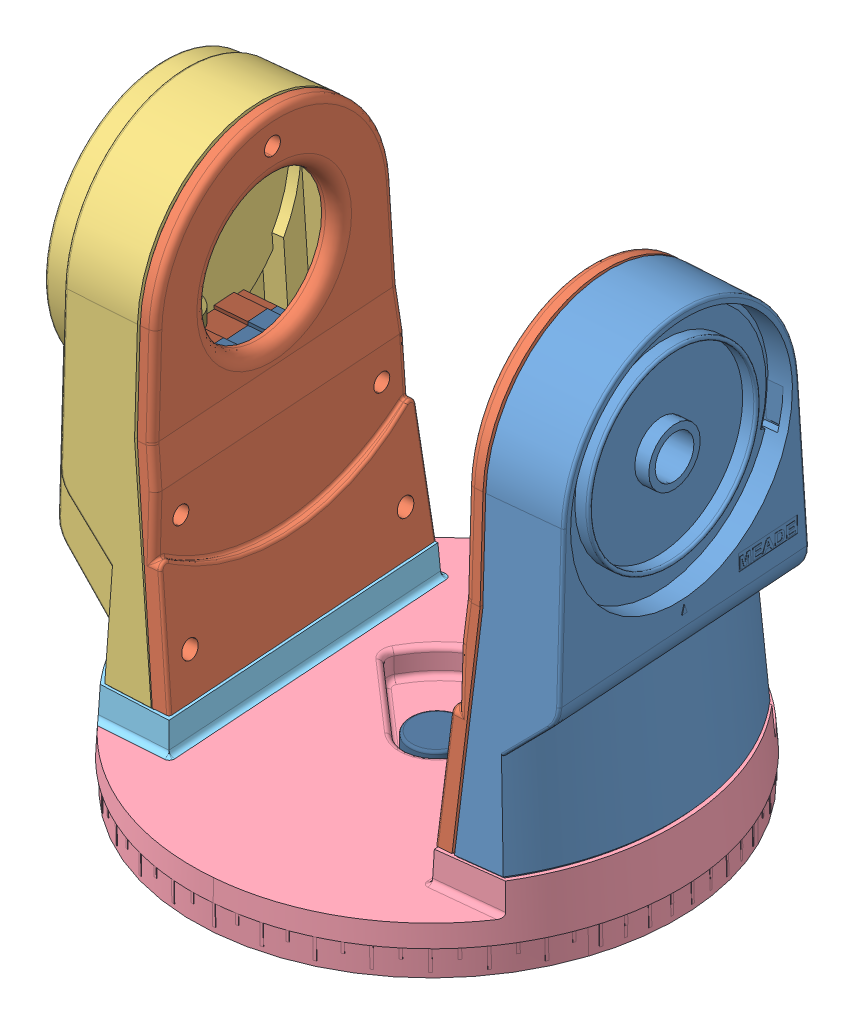
SolidWorks assembly fourche, configuration Défaut. Lengths in mm.
Overall size (198.85 238.33 188.61).
67 component instances, 42 part files, 82 mates.
Components (placement in the parent):
- branche equilibrage-1: branche equilibrage [Défaut] at (-444.0293 45.9192 -837.0232) x (0.999848 0.017413 0.00001) z (0.00001 -0.001172 0.999999) size (42.16 177.75 110.07)
- Plaque carter équilibrage-1: Plaque carter équilibrage [Défaut] at (-443.0317 45.9366 -837.0903) x (0.999848 0.017413 0.00001) z (0.00001 -0.001172 0.999999) size (27.56 165.18 109.18)
- Plaque carter équilibrage-2: Plaque carter équilibrage [Défaut] at (-468.0617 45.0668 -480.7137) x (-0.999848 -0.017413 -0.00001) z (-0.00001 0.001172 -0.999999) size (27.56 165.18 109.18)
- branche motorisée-1: branche motorisée [Défaut] at (-441.716 45.9434 -837.1795) x (0.999848 0.017413 0.00001) z (0.00001 -0.001172 0.999999) size (49.59 177.72 110.04)
- PIED DE fourche-1: PIED DE fourche [Défaut] at (-454.4692 -14.4541 -658.8869) x (0.999848 0.017413 0.00001) z (0.00001 -0.001172 0.999999) size (191.94 35.1 188.57)
  - Pied de fourche-1: Pied de fourche [Défaut] at (12.1809 59.9857 -178.2534) size (191.94 35.1 188.57)
  - Pied de fourche1-1: Pied de fourche1 [Défaut] at (-12.1809 59.9857 178.0188) x (-1 0 0) z (0 0 -1) size (54.8 35.1 115.86)
- rondelle vis m8_50-1: rondelle vis m8_50 [Défaut] at (-454.2843 -25.0712 -659.0167) x (0.997592 0.017452 -0.067129) z (0.017413 -0.999848 -0.001172) size (26.8 26.16 7)
- VisHM8_50-1: VisHM8_50 [Défaut] at (-454.3818 -19.4721 -659.0102) x (0.997592 0.017452 -0.067129) z (0.017413 -0.999848 -0.001172) size (12.6 14.55 55.47)
- limiteur de couple embase-1: limiteur de couple embase [Défaut] at (-453.5008 -70.0544 -659.0694) x (0.06714 0 0.997744) z (-0.997592 -0.017452 0.067129) size (25.3 5 25.3)
- Roue à denture hélicoïdale m=0,5 Z=60-1: Roue à denture hélicoïdale m=0,5 Z=60 [Défaut] at (-453.6431 -61.8856 -659.0599) x (0.201032 0.002353 0.979582) z (-0.017413 0.999848 0.001172) size (31.07 31.07 6.34)
- Levier de débrayage-1: Levier de débrayage [Défaut] at (-491.4971 43.1006 -833.8173) x (0.963244 0.01709 -0.268082) z (0.268062 0.003539 0.963395) size (36.12 10 38.96)
- plateau-1: plateau [Défaut] at (-454.3861 -19.2221 -659.0099) x (-0.997592 -0.017452 0.067129) z (0.017413 -0.999848 -0.001172) size (170 170 47)
- EcrouHM 20-2: EcrouHM 20 [Défaut] at (-453.9456 -44.5183 -659.0395) x (0.06714 0 0.997744) z (-0.017413 0.999848 0.001172) size (30 34.64 12)
- motoreducteur fourche-1: motoreducteur fourche [Défaut] at (-542.1299 45.8782 -641.824) x (0.06714 0 0.997744) z (0.997592 0.017452 -0.067129) size (70.5 139.71 33.06)
  - rep. 01 pignon arbre moteur + disque-1: rep. 01 pignon arbre moteur + disque [Défaut] at (0 -0.36 0) size (19 10.8 19)
  - rep. 02-03 roue Z56-1: rep. 02-03 roue Z56 [Défaut] at (0.8779 -0.6486 0.8082) x (0.995701 0 0.092628) z (-0.092628 0 0.995701) size (28.76 10.95 28.76)
  - rep. 08-09 roue inter-1: rep. 08-09 roue inter [Défaut] at (-0.15 -0.2381 0) x (1 0 0) z (0 0 1) size (12.96 5.74 12.96)
  - rep. 06-07 roue inter-1: rep. 06-07 roue inter [Défaut] at (-0.15 -0.0981 0) x (1 0 0) z (0 0 1) size (13 5.74 13)
  - rep. 04-05 roue inter-1: rep. 04-05 roue inter [Défaut] at (-21.6079 -0.6386 5.1059) x (0.907401 0 -0.420265) z (0.420265 0 0.907401) size (13 5.74 13)
  - bati-1: bati [Défaut] at (103.3128 129.885 -87.3106) size (70.5 138.91 24)
    - Axe Rep19bis-1: Axe Rep19bis [Défaut] at (-92.1856 -130.245 98.2871) x (-0.137137 0 0.990552) z (-0.990552 0 -0.137137) size (3 14 3)
    - moteur-1: moteur [Défaut] at (-103.3128 -129.885 87.3106) size (18 46.5 24)
    - axe-1: axe [Défaut] at (-111.605 -120.0821 97.7106) x (0.934599 0 -0.355704) z (0 -1 0) size (3 3 39)
    - bati2-1: bati2 [Défaut] at (-77.4849 -277.8736 138.6581) x (1 0 0) z (0 0 -1) size (17.4 55.11 17.4)
      - rondelle alu-1: rondelle alu [Défaut] at (-55.9783 -35.2009 30.6529) size (17.4 2.5 17.4)
      - Rondelle M6_1-1: Rondelle M6_1 [Défaut] at (-55.9783 -35.2009 30.6529) size (16.67 2.55 16.67)
      - rondelle alu_1-1: rondelle alu_1 [Défaut] at (-55.9783 -35.2009 30.6529) size (17.4 2.5 17.4)
      - Entretoise_1-1: Entretoise_1 [Défaut] at (-55.9783 -35.2009 30.6529) size (16.5 6 16.5)
      - Entretoise-1: Entretoise [Défaut] at (-55.9783 -35.2009 30.6529) size (16.5 6 16.5)
      - Rondelle M6-1: Rondelle M6 [Défaut] at (-55.9783 -35.2009 30.6529) size (16.67 2.55 16.67)
      - rep. 16 Ecrou M6-1: rep. 16 Ecrou M6 [Défaut] at (18.5294 -120.4752 48.0628) x (-0.896454 0 -0.443136) z (-0.443136 0 0.896454) size (12.68 6 11.39)
    - corps1-1: corps1 [Défaut] at (-126.5989 -147.7633 97.7106) size (62.7 74.5 12)
    - corps2-1: corps2 [Défaut] at (-126.5989 -147.7633 85.7106) size (62.7 50 12)
    - châpe en alu-1: châpe en alu [Défaut] at (-133.4632 -157.3984 87.2051) size (33.3 38 19.61)
  - vis-1: vis [Défaut] at (7.3554 -71.4832 9.6533) x (1 0 0) z (0 1 0) size (33.09 33.06 82.71)
    - Vis san fin m=0,5 - 1 filet(s)-2: Vis san fin m=0,5 - 1 filet(s) [Défaut] at (-0.6479 -0.6412 0.3804) x (0.7262 -0.687484 0) z (0 0 1) size (8.16 8.16 68.9)
    - rep12-4: rep12 [Défaut] at (-11.6724 36.0347 43.7266) x (0.537117 -0.843508 0) z (-0.843508 -0.537117 0) size (23.91 29.81 24)
  - engrenage-1: engrenage [Défaut] at (-45.9983 -125.8694 31.0757) x (-0.919401 0 0.393321) z (0.393321 0 0.919401) size (12.99 17.44 12.99)
    - rep.11SLDPRT-1: rep.11SLDPRT [Défaut] at (-64.557 -106.8565 -14.5787) size (9.52 16 9.52)
    - rep. yacine-1: rep. yacine [Défaut] at (-64.557 -106.8565 -14.5787) size (12.99 1.44 12.99)
  - Vis à tête cylindrique à six pans creux Chc M2,5 - 8-1: Vis à tête cylindrique à six pans creux Chc M2,5 - 8 [Défaut] at (6.7074 -20.6971 10.2945) x (0.636786 0 0.771041) z (0 -1 0) size (4.2 4.2 10.57)
  - joint 9 5 emb-1: joint 9 5 emb [Défaut] at (6.7074 -89.1506 10.2945) size (13.5 2 13.5)
  - joint 9 5 emb-2: joint 9 5 emb [Défaut] at (6.7074 -53.1506 10.2945) size (13.5 2 13.5)
- Vis sans tête à six pans creux à bout cuvette M3 - 3-1: Vis sans tête à six pans creux à bout cuvette M3 - 3 [Réaliste] at (-445.1418 -17.1499 -659.6319) x (-0.019293 -0.859815 -0.51024) z (0.066624 -0.510307 0.857408) size (3.03 3.08 3.04)
- Vis à tête cylindrique bombée cruciforme type H M3 - 10-1: Vis à tête cylindrique bombée cruciforme type H M3 - 10 [Filetage Réaliste] at (-521.841 56.7793 -695.504) x (-0.997592 -0.017452 0.067129) z (-0.0364 0.955572 -0.292501) size (12.58 5.6 5.6)
- Vis à tête cylindrique bombée cruciforme type H M3 - 10-2: Vis à tête cylindrique bombée cruciforme type H M3 - 10 [Filetage Réaliste] at (-508.9533 16.8988 -611.179) x (-0.997592 -0.017452 0.067129) z (-0.040277 -0.642181 -0.765494) size (12.58 5.6 5.6)
- Vis à tête cylindrique bombée cruciforme type H M3 - 10-3: Vis à tête cylindrique bombée cruciforme type H M3 - 10 [Filetage Réaliste] at (-514.8616 16.8988 -698.9804) x (-0.997592 -0.017452 0.067129) z (-0.068087 0.06176 -0.995766) size (12.58 5.6 5.6)
- Vis à tête cylindrique bombée cruciforme type H M3 - 10-4: Vis à tête cylindrique bombée cruciforme type H M3 - 10 [Filetage Réaliste] at (-521.2936 154.7556 -654.4481) x (-0.997592 -0.017452 0.067129) z (-0.06714 0 -0.997744) size (12.58 5.6 5.6)
- Vis à tête cylindrique bombée cruciforme type H M3 - 10-5: Vis à tête cylindrique bombée cruciforme type H M3 - 10 [Filetage Réaliste] at (-516.3356 56.7793 -613.689) x (-0.997592 -0.017452 0.067129) z (-0.06714 0 -0.997744) size (12.58 5.6 5.6)
- Vis à tête cylindrique bombée cruciforme type H M3 - 10-7: Vis à tête cylindrique bombée cruciforme type H M3 - 10 [Filetage Réaliste] at (-393.6444 157.0051 -663.0973) x (0.997592 0.017452 -0.067129) z (0.06714 0 0.997744) size (12.58 5.6 5.6)
- Vis à tête cylindrique bombée cruciforme type H M3 - 10-8: Vis à tête cylindrique bombée cruciforme type H M3 - 10 [Filetage Réaliste] at (-401.1787 18.9039 -706.6898) x (0.997592 0.017452 -0.067129) z (0.06714 0 0.997744) size (12.58 5.6 5.6)
- Vis à tête cylindrique bombée cruciforme type H M3 - 10-10: Vis à tête cylindrique bombée cruciforme type H M3 - 10 [Filetage Réaliste] at (-395.1895 59.0113 -704.086) x (0.997592 0.017452 -0.067129) z (0.06714 0 0.997744) size (12.58 5.6 5.6)
- Vis à tête cylindrique fendue CS M4 - 10-1: Vis à tête cylindrique fendue CS M4 - 10 [Défaut] at (-539.7157 125.5672 -628.3483) x (0.067415 -0.016315 0.997592) z (-0.997592 -0.017452 0.067129) size (7 7 10.62)
- Vis à tête cylindrique fendue CS M4 - 10-2: Vis à tête cylindrique fendue CS M4 - 10 [Défaut] at (-538.2089 116.0774 -615.8713) x (0.067415 -0.016315 0.997592) z (-0.997592 -0.017452 0.067129) size (7 7 10.62)
- Vis à tête cylindrique fendue CS M4 - 10-3: Vis à tête cylindrique fendue CS M4 - 10 [Défaut] at (-539.3849 106.5701 -628.3705) x (0.067415 -0.016315 0.997592) z (-0.997592 -0.017452 0.067129) size (7 7 10.62)
- Vis à tête cylindrique bombée cruciforme type H M3 - 12-2: Vis à tête cylindrique bombée cruciforme type H M3 - 12 [Filetage Réaliste] at (-395.2704 18.9039 -618.8883) x (0.997592 0.017452 -0.067129) z (0.067129 0.000586 0.997744) size (14.59 5.6 5.6)
- Vis à tête cylindrique bombée cruciforme type H M3 - 12-3: Vis à tête cylindrique bombée cruciforme type H M3 - 12 [Filetage Réaliste] at (-389.684 59.0113 -622.271) x (0.997592 0.017452 -0.067129) z (0.068185 -0.42423 0.902984) size (14.59 5.6 5.6)
- Vis à tête cylindrique bombée cruciforme type H M3 - 25-1: Vis à tête cylindrique bombée cruciforme type H M3 - 25 [Filetage Réaliste] at (-516.5693 58.6063 -628.1014) x (-0.997592 -0.017452 0.067129) z (-0.067129 0.486457 -0.871122) size (32.61 5.6 5.6)
- Vis à tête cylindrique bombée cruciforme type H M3 - 25-2: Vis à tête cylindrique bombée cruciforme type H M3 - 25 [Filetage Réaliste] at (-520.3322 72.7741 -680.3366) x (-0.997592 -0.017452 0.067129) z (-0.067129 0.486457 -0.871122) size (32.61 5.6 5.6)
- Vis à tête cylindrique bombée cruciforme type H M3 - 25-3: Vis à tête cylindrique bombée cruciforme type H M3 - 25 [Filetage Réaliste] at (-519.8272 43.7786 -680.3706) x (-0.997592 -0.017452 0.067129) z (0.067053 0.00493 0.997737) size (32.61 5.6 5.6)
- Vis à tête cylindrique bombée cruciforme type H M3 - 20-1: Vis à tête cylindrique bombée cruciforme type H M3 - 20 [Filetage Réaliste] at (-531.1265 -25.9655 -653.8459) x (-0.017413 0.999848 0.001172) z (0.998816 0.017342 0.045444) size (22.61 5.6 5.6)
- Vis à tête cylindrique bombée cruciforme type H M3 - 20-2: Vis à tête cylindrique bombée cruciforme type H M3 - 20 [Filetage Réaliste] at (-512.8439 -25.695 -612.9812) x (-0.017413 0.999848 0.001172) z (0.998816 0.017342 0.045444) size (22.61 5.6 5.6)
- Vis à tête cylindrique bombée cruciforme type H M3 - 20-3: Vis à tête cylindrique bombée cruciforme type H M3 - 20 [Filetage Réaliste] at (-517.7505 -25.6821 -696.841) x (-0.017413 0.999848 0.001172) z (0.998816 0.017342 0.045444) size (22.61 5.6 5.6)
- Vis à tête cylindrique bombée cruciforme type H M3 - 20-4: Vis à tête cylindrique bombée cruciforme type H M3 - 20 [Filetage Réaliste] at (-395.7403 -23.5476 -705.0512) x (-0.017413 0.999848 0.001172) z (0.998816 0.017342 0.045444) size (22.61 5.6 5.6)
- Vis à tête cylindrique bombée cruciforme type H M3 - 20-5: Vis à tête cylindrique bombée cruciforme type H M3 - 20 [Filetage Réaliste] at (-377.4577 -23.2771 -664.1865) x (-0.017413 0.999848 0.001172) z (0.998816 0.017342 0.045444) size (22.61 5.6 5.6)
- Vis à tête cylindrique bombée cruciforme type H M3 - 20-6: Vis à tête cylindrique bombée cruciforme type H M3 - 20 [Filetage Réaliste] at (-390.8337 -23.5604 -621.1914) x (-0.017413 0.999848 0.001172) z (0.998816 0.017342 0.045444) size (22.61 5.6 5.6)
Mates (geometry in assembly coordinates):
- Coïncidente2: coincident anti-aligned: plane of branche equilibrage-1 through (-369.0099 3.4762 -719.0226) normal (0.034821 -0.999391 -0.002343); plane of PIED DE fourche-1/Pied de fourche-1 through (-361.0465 3.5004 -611.0232) normal (-0.034821 0.999391 0.002343)
- Coaxiale4: concentric anti-aligned: cylinder of branche equilibrage-1 through (-391.0008 157.0513 -663.2752) axis (-0.997592 -0.017452 0.067129) radius 1.25; cylinder of Plaque carter équilibrage-1 through (-402.4136 156.8517 -662.5072) axis (0.997592 0.017452 -0.067129) radius 1.5
- Coïncidente10: coincident anti-aligned: plane of branche equilibrage-1 through (-397.0052 121.4404 -709.6249) normal (-0.997592 -0.017452 0.067129); plane of Plaque carter équilibrage-1 through (-408.418 121.5329 -879.2025) normal (0.997592 0.017452 -0.067129)
- Parallèle1: parallel aligned: plane of branche equilibrage-1 through (-369.0099 3.4762 -719.0226) normal (0.034821 -0.999391 -0.002343); plane of Plaque carter équilibrage-1 through (-422.1214 1.9816 -878.2804) normal (0.034821 -0.999391 -0.002343)
- Coaxiale9: concentric anti-aligned: cone of Plaque carter équilibrage-2 through (-509.6865 154.9588 -655.2893) axis (-0.997592 -0.017452 0.067129); cylinder of branche motorisée-1 through (-524.1906 154.705 -654.3133) axis (0.997592 0.017452 -0.067129) radius 1.25
- Coïncidente13: coincident anti-aligned: plane of Plaque carter équilibrage-2 through (-505.285 119.3131 -438.4259) normal (-0.997592 -0.017452 0.067129); plane of branche motorisée-1 through (-516.6997 119.2197 -608.081) normal (0.997592 0.017452 -0.067129)
- Coïncidente21: coincident: line of Plaque carter équilibrage-1 through (-403.9093 2.9849 -608.7792) axis (-0.06714 0 -0.997744); plane of PIED DE fourche-1/Pied de fourche-1 through (-403.8836 2.0012 -608.1406) normal (-0.997592 0.017452 0.067129)
- Coïncidente30: coincident: plane of Plaque carter équilibrage-1; line of PIED DE fourche-1/Pied de fourche1-1 through (-454.3978 -18.553 -659.0091) axis (0.017413 -0.999848 -0.001172)
- Coïncidente34: coincident: line of Plaque carter équilibrage-2 through (-679.7698 -1.6347 -696.1892) axis (0.067167 -0.001579 0.99774); plane of PIED DE fourche-1/Pied de fourche1-1 through (-505.5991 0.3489 -709.8313) normal (0.996376 0.052336 -0.067048)
- Coaxiale10: concentric anti-aligned: cylinder of rondelle vis m8_50-1 through (-454.2599 -26.471 -659.0184) axis (-0.017413 0.999848 0.001172) radius 4.1; cylinder of VisHM8_50-1 through (-454.3818 -19.4721 -659.0102) axis (0.017413 -0.999848 -0.001172) radius 4
- Coaxiale11: concentric aligned: cylinder of PIED DE fourche-1/Pied de fourche-1 through (-454.4758 -14.0729 -659.0038) axis (0.017413 -0.999848 -0.001172) radius 5.4; cylinder of VisHM8_50-1 through (-454.3818 -19.4721 -659.0102) axis (0.017413 -0.999848 -0.001172) radius 4
- Coïncidente52: coincident anti-aligned: plane of rondelle vis m8_50-1 through (-454.3818 -19.4721 -659.0102) normal (-0.017413 0.999848 0.001172); plane of VisHM8_50-1 through (-447.8527 -19.3621 -655.804) normal (0.017413 -0.999848 -0.001172)
- Parallèle2: parallel aligned: plane of rondelle vis m8_50-1 through (-450.1698 -26.3995 -659.2936) normal (-0.997592 -0.017452 0.067129); plane of VisHM8_50-1 through (-450.6882 -24.4364 -635.2044) normal (-0.997592 -0.017452 0.067129)
- Coïncidente54: coincident anti-aligned: plane of PIED DE fourche-1/Pied de fourche-1 through (-454.2843 -25.0712 -659.0167) normal (0.017413 -0.999848 -0.001172); plane of rondelle vis m8_50-1 through (-454.2843 -25.0712 -659.0167) normal (-0.017413 0.999848 0.001172)
- Parallèle3: parallel: line of PIED DE fourche-1/Pied de fourche1-1 through (-497.7587 -8.9641 -600.586) axis (-0.06714 0 -0.997744); plane of rondelle vis m8_50-1 through (-458.35 -26.5426 -658.7431) normal (0.997592 0.017452 -0.067129)
- Coïncidente56: coincident anti-aligned: plane of Levier de débrayage-1 through (-454.3713 -20.072 -659.0109) normal (0.017413 -0.999848 -0.001172); plane of PIED DE fourche-1/Pied de fourche-1 through (-425.2551 -19.5401 -680.176) normal (-0.017413 0.999848 0.001172)
- Parallèle4: parallel anti-aligned: plane of VisHM8_50-1 through (-454.9625 -14.1729 -666.2621) normal (0.440651 0.008726 -0.897636); plane of Levier de débrayage-1 through (-455.3417 6.7117 -666.4681) normal (-0.440651 -0.008726 0.897636)
- Coïncidente61: coincident anti-aligned: plane of limiteur de couple embase-1 through (-454.4372 -65.0551 -671.685) normal (-0.017413 0.999848 0.001172); plane of Roue à denture hélicoïdale m=0,5 Z=60-1 through (-453.5879 -65.0551 -659.0636) normal (0.017413 -0.999848 -0.001172)
- Coaxiale20: concentric aligned: cylinder of limiteur de couple embase-1 through (-453.5008 -70.0544 -659.0694) axis (0.017413 -0.999848 -0.001172) radius 12.65; cylinder of Roue à denture hélicoïdale m=0,5 Z=60-1 through (-453.6983 -58.7161 -659.0561) axis (0.017413 -0.999848 -0.001172) radius 6.85
- Coaxiale21: concentric aligned: cylinder of VisHM8_50-1 through (-454.3818 -19.4721 -659.0102) axis (0.017413 -0.999848 -0.001172) radius 4; cylinder of limiteur de couple embase-1 through (-453.5008 -70.0544 -659.0694) axis (0.017413 -0.999848 -0.001172) radius 3.4
- Coaxiale22: concentric anti-aligned: cylinder of VisHM8_50-1 through (-454.3818 -19.4721 -659.0102) axis (0.017413 -0.999848 -0.001172) radius 4; cylinder of plateau-1 through (-454.3339 -22.2217 -659.0134) axis (-0.017413 0.999848 0.001172) radius 85
- Distance1: distance = 1 mm anti-aligned: plane of plateau-1 through (-454.441 -16.0726 -659.0062) normal (-0.017413 0.999848 0.001172); plane of PIED DE fourche-1/Pied de fourche-1 through (-377.624 -13.7286 -664.1753) normal (0.017413 -0.999848 -0.001172)
- Coïncidente64: coincident aligned: plane of PIED DE fourche-1/Pied de fourche-1; plane of plateau-1
- Parallèle5: parallel anti-aligned: plane of limiteur de couple embase-1 through (-441.0163 -66.7384 -657.4039) normal (-0.06714 0 -0.997744); plane of plateau-1 through (-456.7222 -64.2727 -656.3721) normal (0.06714 0 0.997744)
- Parallèle9: parallel anti-aligned: plane of branche motorisée-1 through (-539.5714 0.3489 -599.0106) normal (0 -1 0); plane of PIED DE fourche-1/Pied de fourche1-1 through (-548.4623 0.3489 -706.947) normal (0 1 0)
- Coïncidente80: coincident: point of branche motorisée-1; line of PIED DE fourche-1/Pied de fourche1-1 through (-531.345 -13.4174 -653.8312) axis (0.017413 -0.999848 -0.001172)
- Coaxiale35: concentric anti-aligned: cylinder of VisHM8_50-1 through (-454.3818 -19.4721 -659.0102) axis (0.017413 -0.999848 -0.001172) radius 4; cone of Levier de débrayage-1 through (-454.5455 -10.0735 -658.9991) axis (-0.017413 0.999848 0.001172)
- Coïncidente82: coincident anti-aligned: plane of rondelle vis m8_50-1 through (-454.2599 -26.471 -659.0184) normal (0.017413 -0.999848 -0.001172); plane of plateau-1 through (-454.2599 -26.471 -659.0184) normal (-0.017413 0.999848 0.001172)
- Coïncidente83: coincident anti-aligned: plane of Roue à denture hélicoïdale m=0,5 Z=60-1 through (-453.6983 -58.7161 -659.0561) normal (-0.017413 0.999848 0.001172); plane of plateau-1 through (-453.6983 -58.7161 -659.0561) normal (0.017413 -0.999848 -0.001172)
- Parallèle11: parallel aligned: line of Plaque carter équilibrage-2 through (-505.674 1.314 -709.1265) axis (0.06714 0 0.997744); line of PIED DE fourche-1/Pied de fourche1-1 through (-505.6487 0.3489 -710.5673) axis (0.06714 0 0.997744)
- Coaxiale23: concentric anti-aligned: cylinder of VisHM8_50-1 through (-454.3818 -19.4721 -659.0102) axis (0.017413 -0.999848 -0.001172) radius 4; cylinder of EcrouHM 20-2 through (-453.7366 -56.5164 -659.0536) axis (-0.017413 0.999848 0.001172) radius 10
- Perpendiculaire1: perpendicular: plane of Plaque carter équilibrage-2 through (-510.8056 116.9333 -655.1538) normal (0.997592 0.017452 -0.067129); plane of EcrouHM 20-2 through (-461.3689 -56.6676 -643.5061) normal (0.06714 0 0.997744)
- Parallèle12: parallel anti-aligned: plane of plateau-1 through (-454.3339 -22.2217 -659.0134) normal (0.017413 -0.999848 -0.001172); plane of motoreducteur fourche-1/bati-1/châpe en alu-1 through (-541.8121 135.0238 -621.2916) normal (-0.017413 0.999848 0.001172)
- Coaxiale16: concentric anti-aligned: cylinder of branche motorisée-1 through (-542.1099 125.5253 -628.1871) axis (0.997592 0.017452 -0.067129) radius 1.25; cylinder of motoreducteur fourche-1/bati-1/châpe en alu-1 through (-522.5571 125.8673 -629.5029) axis (-0.997592 -0.017452 0.067129) radius 2.15
- Coïncidente99: coincident anti-aligned: plane of branche motorisée-1 through (-541.7791 106.5282 -628.2094) normal (0.997592 0.017452 -0.067129); plane of motoreducteur fourche-1/bati-1/châpe en alu-1 through (-541.4391 97.0296 -625.6264) normal (-0.997592 -0.017452 0.067129)
- Coaxiale15: concentric anti-aligned: cylinder of Levier de débrayage-1 through (-447.935 -17.1987 -659.444) axis (-0.997592 -0.017452 0.067129) radius 1.25; cylinder of Vis sans tête à six pans creux à bout cuvette M3 - 3-1 through (-445.1418 -17.1499 -659.6319) axis (0.997592 0.017452 -0.067129) radius 1.5
- Coïncidente97: coincident aligned: plane of VisHM8_50-1 through (-448.4334 -14.0629 -663.056) normal (0.997592 0.017452 -0.067129); circle of Vis sans tête à six pans creux à bout cuvette M3 - 3-1
- Coaxiale36: concentric anti-aligned: cone of Plaque carter équilibrage-2 through (-510.7287 56.9737 -696.2517) axis (-0.997592 -0.017452 0.067129); cylinder of Vis à tête cylindrique bombée cruciforme type H M3 - 10-1 through (-521.841 56.7793 -695.504) axis (0.997592 0.017452 -0.067129) radius 2.8
- Coïncidente107: coincident anti-aligned: plane of Plaque carter équilibrage-2 through (-524.0736 54.2581 -693.5848) normal (0.997592 0.017452 -0.067129); plane of Vis à tête cylindrique bombée cruciforme type H M3 - 10-1 through (-524.2353 56.7374 -695.3428) normal (-0.997592 -0.017452 0.067129)
- Coaxiale37: concentric anti-aligned: cone of Plaque carter équilibrage-2 through (-500.5661 17.0456 -611.7433) axis (-0.997592 -0.017452 0.067129); cylinder of Vis à tête cylindrique bombée cruciforme type H M3 - 10-2 through (-508.9533 16.8988 -611.179) axis (0.997592 0.017452 -0.067129) radius 2.8
- Coïncidente106: coincident anti-aligned: plane of Plaque carter équilibrage-2 through (-511.1798 14.2852 -609.1943) normal (0.997592 0.017452 -0.067129); plane of Vis à tête cylindrique bombée cruciforme type H M3 - 10-2 through (-511.3475 16.8569 -611.0178) normal (-0.997592 -0.017452 0.067129)
- Coaxiale19: concentric anti-aligned: cone of Plaque carter équilibrage-2 through (-506.4744 17.0456 -699.5448) axis (-0.997592 -0.017452 0.067129); cylinder of Vis à tête cylindrique bombée cruciforme type H M3 - 10-3 through (-514.8616 16.8988 -698.9804) axis (0.997592 0.017452 -0.067129) radius 2.8
- Coïncidente102: coincident anti-aligned: plane of Plaque carter équilibrage-2 through (-517.0881 14.2852 -696.9958) normal (0.997592 0.017452 -0.067129); plane of Vis à tête cylindrique bombée cruciforme type H M3 - 10-3 through (-517.2558 16.8569 -698.8193) normal (-0.997592 -0.017452 0.067129)
- Coïncidente108: coincident anti-aligned: plane of Plaque carter équilibrage-2 through (-523.7885 154.7138 -655.7836) normal (0.997592 0.017452 -0.067129); plane of Vis à tête cylindrique bombée cruciforme type H M3 - 10-4 through (-523.6878 154.7138 -654.287) normal (-0.997592 -0.017452 0.067129)
- Coaxiale38: concentric anti-aligned: cone of Plaque carter équilibrage-2 through (-523.6878 154.7138 -654.287) axis (-0.997592 -0.017452 0.067129); cylinder of Vis à tête cylindrique bombée cruciforme type H M3 - 10-4 through (-521.2936 154.7556 -654.4481) axis (0.997592 0.017452 -0.067129) radius 2.8
- Coaxiale24: concentric anti-aligned: cone of Plaque carter équilibrage-2 through (-505.2232 56.9737 -614.4367) axis (-0.997592 -0.017452 0.067129); cylinder of Vis à tête cylindrique bombée cruciforme type H M3 - 10-5 through (-516.3356 56.7793 -613.689) axis (0.997592 0.017452 -0.067129) radius 2.8
- Coïncidente109: coincident anti-aligned: plane of Plaque carter équilibrage-2 through (-518.8051 54.2581 -615.2917) normal (0.997592 0.017452 -0.067129); plane of Vis à tête cylindrique bombée cruciforme type H M3 - 10-5 through (-518.7298 56.7374 -613.5279) normal (-0.997592 -0.017452 0.067129)
- Coaxiale29: concentric anti-aligned: cone of Plaque carter équilibrage-1 through (-391.2502 157.047 -663.2584) axis (0.997592 0.017452 -0.067129); cylinder of Vis à tête cylindrique bombée cruciforme type H M3 - 10-7 through (-393.6444 157.0051 -663.0973) axis (-0.997592 -0.017452 0.067129) radius 2.8
- Coïncidente114: coincident anti-aligned: plane of Plaque carter équilibrage-1 through (-391.1495 157.047 -661.7618) normal (-0.997592 -0.017452 0.067129); plane of Vis à tête cylindrique bombée cruciforme type H M3 - 10-7 through (-391.2502 157.047 -663.2584) normal (0.997592 0.017452 -0.067129)
- Coïncidente111: coincident anti-aligned: plane of Plaque carter équilibrage-1 through (-398.8626 16.3741 -708.6804) normal (-0.997592 -0.017452 0.067129); plane of Vis à tête cylindrique bombée cruciforme type H M3 - 10-8 through (-398.7845 18.9458 -706.8509) normal (0.997592 0.017452 -0.067129)
- Coaxiale26: concentric anti-aligned: cone of Plaque carter équilibrage-1 through (-409.566 18.7572 -706.1254) axis (0.997592 0.017452 -0.067129); cylinder of Vis à tête cylindrique bombée cruciforme type H M3 - 10-8 through (-401.1787 18.9039 -706.6898) axis (-0.997592 -0.017452 0.067129) radius 2.8
- Coaxiale25: concentric anti-aligned: cone of Plaque carter équilibrage-1 through (-406.3018 58.8169 -703.3382) axis (0.997592 0.017452 -0.067129); cylinder of Vis à tête cylindrique bombée cruciforme type H M3 - 10-10 through (-395.1895 59.0113 -704.086) axis (-0.997592 -0.017452 0.067129) radius 2.8
- Coïncidente110: coincident anti-aligned: plane of Plaque carter équilibrage-1 through (-392.6336 56.5738 -702.4891) normal (-0.997592 -0.017452 0.067129); plane of Vis à tête cylindrique bombée cruciforme type H M3 - 10-10 through (-392.7953 59.0532 -704.2471) normal (0.997592 0.017452 -0.067129)
- Coaxiale39: concentric anti-aligned: cylinder of branche motorisée-1 through (-541.1019 116.0267 -615.6766) axis (0.997592 0.017452 -0.067129) radius 1.25; cylinder of Vis à tête cylindrique fendue CS M4 - 10-2 through (-538.2089 116.0774 -615.8713) axis (-0.997592 -0.017452 0.067129) radius 2
- Coïncidente115: coincident anti-aligned: plane of motoreducteur fourche-1/bati-1/châpe en alu-1 through (-536.8565 116.0773 -595.7741) normal (0.997592 0.017452 -0.067129); plane of Vis à tête cylindrique fendue CS M4 - 10-2 through (-538.2089 116.0774 -615.8713) normal (-0.997592 -0.017452 0.067129)
- Coïncidente116: coincident aligned: plane of Vis à tête cylindrique fendue CS M4 - 10-1 through (-539.7157 125.5672 -628.3483) normal (-0.997592 -0.017452 0.067129); plane of Vis à tête cylindrique fendue CS M4 - 10-3 through (-539.3849 106.5701 -628.3705) normal (-0.997592 -0.017452 0.067129)
- Coaxiale40: concentric anti-aligned: cylinder of branche motorisée-1 through (-542.1099 125.5253 -628.1871) axis (0.997592 0.017452 -0.067129) radius 1.25; cylinder of Vis à tête cylindrique fendue CS M4 - 10-1 through (-539.7157 125.5672 -628.3483) axis (-0.997592 -0.017452 0.067129) radius 2
- Coaxiale41: concentric anti-aligned: cylinder of branche motorisée-1 through (-541.7791 106.5282 -628.2094) axis (0.997592 0.017452 -0.067129) radius 1.25; cylinder of Vis à tête cylindrique fendue CS M4 - 10-3 through (-539.3849 106.5701 -628.3705) axis (-0.997592 -0.017452 0.067129) radius 2
- Coïncidente117: coincident anti-aligned: plane of motoreducteur fourche-1/bati-1/châpe en alu-1 through (-539.7832 102.0707 -635.4598) normal (0.997592 0.017452 -0.067129); plane of Vis à tête cylindrique fendue CS M4 - 10-1 through (-539.7157 125.5672 -628.3483) normal (-0.997592 -0.017452 0.067129)
- Coaxiale43: concentric anti-aligned: cylinder of motoreducteur fourche-1/bati-1/corps1-1 through (-518.9635 58.5644 -627.9402) axis (-0.997592 -0.017452 0.067129) radius 1.75; cylinder of Vis à tête cylindrique bombée cruciforme type H M3 - 25-1 through (-516.5693 58.6063 -628.1014) axis (0.997592 0.017452 -0.067129) radius 2.8
- Coïncidente119: coincident anti-aligned: plane of motoreducteur fourche-1/bati-1/corps1-1 through (-522.7264 72.7323 -680.1755) normal (0.997592 0.017452 -0.067129); plane of Vis à tête cylindrique bombée cruciforme type H M3 - 25-1 through (-518.9635 58.5644 -627.9402) normal (-0.997592 -0.017452 0.067129)
- Coaxiale44: concentric anti-aligned: cylinder of motoreducteur fourche-1/bati-1/corps1-1 through (-522.2214 43.7367 -680.2095) axis (-0.997592 -0.017452 0.067129) radius 1.75; cylinder of Vis à tête cylindrique bombée cruciforme type H M3 - 25-3 through (-519.8272 43.7786 -680.3706) axis (0.997592 0.017452 -0.067129) radius 2.8
- Coïncidente120: coincident anti-aligned: plane of motoreducteur fourche-1/bati-1/corps1-1 through (-522.7264 72.7323 -680.1755) normal (0.997592 0.017452 -0.067129); plane of Vis à tête cylindrique bombée cruciforme type H M3 - 25-3 through (-522.2214 43.7367 -680.2095) normal (-0.997592 -0.017452 0.067129)
- Coaxiale45: concentric anti-aligned: cylinder of Vis à tête cylindrique bombée cruciforme type H M3 - 25-2 through (-520.3322 72.7741 -680.3366) axis (0.997592 0.017452 -0.067129) radius 2.8; cylinder of motoreducteur fourche-1/bati-1/corps1-1 through (-522.7264 72.7323 -680.1755) axis (-0.997592 -0.017452 0.067129) radius 1.15
- Coïncidente121: coincident anti-aligned: plane of motoreducteur fourche-1/bati-1/corps1-1 through (-522.7264 72.7323 -680.1755) normal (0.997592 0.017452 -0.067129); plane of Vis à tête cylindrique bombée cruciforme type H M3 - 25-2 through (-522.7264 72.7323 -680.1755) normal (-0.997592 -0.017452 0.067129)
- Coaxiale48: concentric anti-aligned: cone of Plaque carter équilibrage-1 through (-400.7964 58.8169 -621.5233) axis (0.997592 0.017452 -0.067129); cylinder of Vis à tête cylindrique bombée cruciforme type H M3 - 12-3 through (-389.684 59.0113 -622.271) axis (-0.997592 -0.017452 0.067129) radius 2.8
- Coïncidente122: coincident anti-aligned: plane of Plaque carter équilibrage-1 through (-387.3651 56.5738 -624.196) normal (-0.997592 -0.017452 0.067129); plane of Vis à tête cylindrique bombée cruciforme type H M3 - 12-3 through (-387.2898 59.0532 -622.4322) normal (0.997592 0.017452 -0.067129)
- Coaxiale49: concentric anti-aligned: cone of Plaque carter équilibrage-1 through (-403.6577 18.7572 -618.3239) axis (0.997592 0.017452 -0.067129); cylinder of Vis à tête cylindrique bombée cruciforme type H M3 - 12-2 through (-395.2704 18.9039 -618.8883) axis (-0.997592 -0.017452 0.067129) radius 2.8
- Coïncidente123: coincident anti-aligned: plane of Plaque carter équilibrage-1 through (-392.9543 16.3741 -620.879) normal (-0.997592 -0.017452 0.067129); plane of Vis à tête cylindrique bombée cruciforme type H M3 - 12-2 through (-392.8762 18.9458 -619.0494) normal (0.997592 0.017452 -0.067129)
- Coïncidente124: coincident anti-aligned: plane of branche motorisée-1 through (-539.5714 0.3489 -599.0106) normal (0 -1 0); plane of PIED DE fourche-1/Pied de fourche1-1 through (-548.4623 0.3489 -706.947) normal (0 1 0)
- Coïncidente125: coincident anti-aligned: plane of plateau-1 through (-454.3339 -22.2217 -659.0134) normal (0.017413 -0.999848 -0.001172); plane of Vis à tête cylindrique bombée cruciforme type H M3 - 20-1 through (-531.1682 -23.5658 -653.8431) normal (-0.017413 0.999848 0.001172)
- Coaxiale31: concentric aligned: cylinder of plateau-1 through (-531.1682 -23.5658 -653.8431) axis (0.017413 -0.999848 -0.001172) radius 1.7; cylinder of Vis à tête cylindrique bombée cruciforme type H M3 - 20-1 through (-531.1265 -25.9655 -653.8459) axis (0.017413 -0.999848 -0.001172) radius 2.8
- Coaxiale30: concentric aligned: cylinder of plateau-1 through (-512.8857 -23.2953 -612.9784) axis (0.017413 -0.999848 -0.001172) radius 1.7; cylinder of Vis à tête cylindrique bombée cruciforme type H M3 - 20-2 through (-512.8439 -25.695 -612.9812) axis (0.017413 -0.999848 -0.001172) radius 2.8
- Coïncidente126: coincident anti-aligned: plane of plateau-1 through (-454.3339 -22.2217 -659.0134) normal (0.017413 -0.999848 -0.001172); plane of Vis à tête cylindrique bombée cruciforme type H M3 - 20-2 through (-512.8857 -23.2953 -612.9784) normal (-0.017413 0.999848 0.001172)
- Coïncidente118: coincident anti-aligned: plane of plateau-1 through (-454.3339 -22.2217 -659.0134) normal (0.017413 -0.999848 -0.001172); plane of Vis à tête cylindrique bombée cruciforme type H M3 - 20-3 through (-517.7923 -23.2825 -696.8381) normal (-0.017413 0.999848 0.001172)
- Coaxiale32: concentric aligned: cylinder of plateau-1 through (-517.7923 -23.2825 -696.8381) axis (0.017413 -0.999848 -0.001172) radius 1.7; cylinder of Vis à tête cylindrique bombée cruciforme type H M3 - 20-3 through (-517.7505 -25.6821 -696.841) axis (0.017413 -0.999848 -0.001172) radius 2.8
- Coïncidente127: coincident anti-aligned: plane of plateau-1 through (-454.3339 -22.2217 -659.0134) normal (0.017413 -0.999848 -0.001172); plane of Vis à tête cylindrique bombée cruciforme type H M3 - 20-4 through (-395.7821 -21.148 -705.0484) normal (-0.017413 0.999848 0.001172)
- Coaxiale33: concentric aligned: cylinder of plateau-1 through (-395.7821 -21.148 -705.0484) axis (0.017413 -0.999848 -0.001172) radius 1.7; cylinder of Vis à tête cylindrique bombée cruciforme type H M3 - 20-4 through (-395.7403 -23.5476 -705.0512) axis (0.017413 -0.999848 -0.001172) radius 2.8
- Coïncidente128: coincident anti-aligned: plane of plateau-1 through (-454.3339 -22.2217 -659.0134) normal (0.017413 -0.999848 -0.001172); plane of Vis à tête cylindrique bombée cruciforme type H M3 - 20-5 through (-377.4995 -20.8775 -664.1837) normal (-0.017413 0.999848 0.001172)
- Coaxiale34: concentric aligned: cylinder of plateau-1 through (-377.4995 -20.8775 -664.1837) axis (0.017413 -0.999848 -0.001172) radius 1.7; cylinder of Vis à tête cylindrique bombée cruciforme type H M3 - 20-5 through (-377.4577 -23.2771 -664.1865) axis (0.017413 -0.999848 -0.001172) radius 2.8
- Coïncidente129: coincident anti-aligned: plane of plateau-1 through (-454.3339 -22.2217 -659.0134) normal (0.017413 -0.999848 -0.001172); plane of Vis à tête cylindrique bombée cruciforme type H M3 - 20-6 through (-390.8755 -21.1608 -621.1886) normal (-0.017413 0.999848 0.001172)
- Coaxiale50: concentric aligned: cylinder of plateau-1 through (-390.8755 -21.1608 -621.1886) axis (0.017413 -0.999848 -0.001172) radius 1.7; cylinder of Vis à tête cylindrique bombée cruciforme type H M3 - 20-6 through (-390.8337 -23.5604 -621.1914) axis (0.017413 -0.999848 -0.001172) radius 2.8
